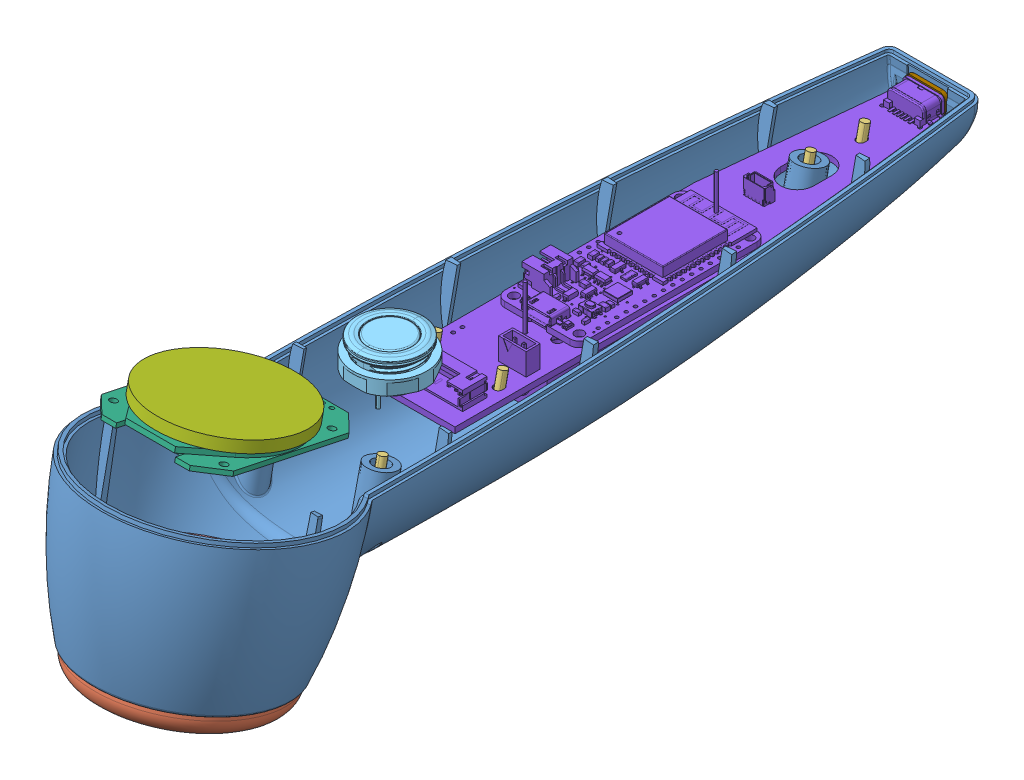
SolidWorks assembly PlasticScannerAssembly, configuration Default. Lengths in mm.
Overall size (62.38 71.41 231.21).
20 component instances, 13 part files, 54 mates.
Components (placement in the parent):
- Bottom shell-1: Bottom shell [Default] at origin size (62.38 51.39 230.69)
- Top Shell-1: Top Shell [Default] at origin size (62 34.67 227.14) (hidden)
- D profile seal ring-1: D profile seal ring [Default] at (0 -28.8554 6.1334) x (-0.032569 0.207801 0.977629) z (0.999469 0.006772 0.031857) size (48 7 48)
- BN_20002_3148566_hexalobular_socket_pan_head_screw_2_2x6-1: BN_20002_3148566_hexalobular_socket_pan_head_screw_2_2x6 [Default] at (-17.145 -14.0085 12.9751) x (0 -0.978148 0.207912) z (-0.651464 -0.157738 -0.7421) size (7.61 4 4)
- BN_20002_3148566_hexalobular_socket_pan_head_screw_2_2x6-2: BN_20002_3148566_hexalobular_socket_pan_head_screw_2_2x6 [Default] at (14.351 -17.7843 -4.7891) x (0 -0.978148 0.207912) z (-0.207912 0.203368 0.956773) size (7.61 4 4)
- PCB KiCad v0.4-1: PCB KiCad v0.4 [Default] at (-0.254 -16.1472 2.9129) x (1 0 0) z (0 -0.978148 0.207912) size (49.12 49.12 11.99)
- Push_buttonSwitch_MCS16_ZNC_ZNC_PIN_02-1: Push_buttonSwitch_MCS16_ZNC_ZNC_PIN_02 [Default] at (0 8.2 -50) size (20 15.41 20)
- BN_20002_3148566_hexalobular_socket_pan_head_screw_2_2x6-3: BN_20002_3148566_hexalobular_socket_pan_head_screw_2_2x6 [Default] at (-16 0.6097 -30.7998) x (0 0.978148 -0.207912) z (-0.207912 -0.203368 -0.956773) size (7.61 4 4)
- BN_20002_3148566_hexalobular_socket_pan_head_screw_2_2x6-4: BN_20002_3148566_hexalobular_socket_pan_head_screw_2_2x6 [Default] at (16 0.6097 -30.7998) x (0 0.978148 -0.207912) z (-0.207912 -0.203368 -0.956773) size (7.61 4 4)
- BN_20002_3148566_hexalobular_socket_pan_head_screw_2_2x6-5: BN_20002_3148566_hexalobular_socket_pan_head_screw_2_2x6 [Default] at (0 -1.9651 -163.1568) x (0 0.978148 -0.207912) z (-0.710006 -0.14641 -0.688807) size (7.61 4 4)
- Screen GC9A01 128 tft-1: Screen GC9A01 128 tft [Default] at (0 21.3737 -5.2588) x (1 0 0) z (0 0.207912 0.978148) size (36 2.7 44)
- 3mm glass-1: 3mm glass [Default] at (0 22.9865 -4.8859) x (0.980992 0.040345 0.189807) z (-0.194047 0.20396 0.959555) size (38 3 38)
- ControllerBoard -02-12-2022-2: ControllerBoard -02-12-2022 [Default] at (110.65 -2.1 -20.2) x (-1 0 0) z (0 1 0) size (25 142.1 26.9)
- CX60-24S-1000-C--3DModel-STEP-1-1: CX60-24S-1000-C--3DModel-STEP-1 [Default] at (4.05 7.135 -1179.513) x (0 0 1) z (0 -1 0) size (1000.01 12.36 6.51) (hidden)
- USB gasket-1: USB gasket [Default] at (0 1.25 -196.9) size (11 5.5 1.5)
- Lower glass-1: Lower glass [Default] at (0 -23.4755 4.9899) x (1 0 0) z (0 0.207912 0.978148) size (25 2 25)
- Lower O ring-1: Lower O ring [Default] at (0 -21.3236 4.5325) x (0.999365 0.007406 0.034843) z (-0.035621 0.20778 0.977527) size (25 8.31 25)
- BN_20002_3148566_hexalobular_socket_pan_head_screw_2_2x6-6: BN_20002_3148566_hexalobular_socket_pan_head_screw_2_2x6 [Default] at (0 -2.5158 -177.8637) x (0 0.978148 -0.207912) z (-0.710006 -0.14641 -0.688807) size (7.61 4 4)
- BN_20002_3148566_hexalobular_socket_pan_head_screw_2_2x6-7: BN_20002_3148566_hexalobular_socket_pan_head_screw_2_2x6 [Default] at (9 -2.5158 -70.5179) x (0 0.978148 -0.207912) z (-0.710006 -0.14641 -0.688807) size (7.61 4 4)
- BN_20002_3148566_hexalobular_socket_pan_head_screw_2_2x6-8: BN_20002_3148566_hexalobular_socket_pan_head_screw_2_2x6 [Default] at (-9 -2.5158 -70.5179) x (0 0.978148 -0.207912) z (-0.710006 -0.14641 -0.688807) size (7.61 4 4)
Mates (geometry in assembly coordinates):
- Coincident1: coincident aligned: plane of Bottom shell-1 through (0 0 0) normal (0 0 1)
- Coincident2: coincident aligned: plane of Top Shell-1 through (0 0 0) normal (0 0 1)
- Coincident3: coincident aligned: plane of Bottom shell-1 through (0 0 0) normal (0 1 0)
- Coincident4: coincident aligned: plane of Top Shell-1 through (0 0 0) normal (0 1 0)
- Coincident5: coincident aligned: plane of Bottom shell-1 through (0 0 0) normal (1 0 0)
- Coincident6: coincident aligned: plane of Top Shell-1 through (0 0 0) normal (1 0 0)
- Concentric5: concentric aligned: cone of Bottom shell-1 through (-17.145 -16.5516 13.5156) axis (0 -0.978148 0.207912); cylinder of BN_20002_3148566_hexalobular_socket_pan_head_screw_2_2x6-1 through (-17.145 -19.8773 14.2225) axis (0 -0.978148 0.207912) radius 1.1
- Concentric7: concentric anti-aligned: circle of Bottom shell-1; circle of PCB KiCad v0.4-1
- Concentric8: concentric aligned: cylinder of BN_20002_3148566_hexalobular_socket_pan_head_screw_2_2x6-2 through (14.351 -23.6532 -3.5416) axis (0 -0.978148 0.207912) radius 1.1; circle of PCB KiCad v0.4-1
- Coincident13: coincident anti-aligned: plane of Bottom shell-1 through (0 -19.3494 -4.4564) normal (0 0.978148 -0.207912); plane of PCB KiCad v0.4-1 through (0 -17.6067 3.7424) normal (0 -0.978148 0.207912)
- Coincident14: coincident anti-aligned: circle of BN_20002_3148566_hexalobular_socket_pan_head_screw_2_2x6-2; plane of PCB KiCad v0.4-1 through (0 -16.0416 3.4098) normal (0 0.978148 -0.207912)
- Coincident15: coincident anti-aligned: circle of BN_20002_3148566_hexalobular_socket_pan_head_screw_2_2x6-1; plane of PCB KiCad v0.4-1 through (0 -16.0416 3.4098) normal (0 0.978148 -0.207912)
- Concentric9: concentric anti-aligned: circle of Bottom shell-1; circle of PCB KiCad v0.4-1
- Concentric11: concentric aligned: cylinder of Bottom shell-1 through (0 -34.3669 36.4416) axis (0 0.978148 -0.207912) radius 1.15; cylinder of BN_20002_3148567_hexalobular_socket_pan_head_screw_2_2x8-1 through (0 20.1086 24.8625) axis (0 0.978148 -0.207912) radius 1.1
- Coincident18: coincident anti-aligned: plane of Bottom shell-1 through (0 6.358 -1.3514) normal (0 -0.978148 0.207912); circle of BN_20002_3148567_hexalobular_socket_pan_head_screw_2_2x8-1
- Distance1: distance = 0.5 mm anti-aligned: plane of Top Shell-1 through (0 16.5 0) normal (0 1 0); plane of Push_buttonSwitch_MCS16_ZNC_ZNC_PIN_02-1 through (0 17 -58) normal (0 -1 0)
- Coincident24: coincident aligned: plane of Push_buttonSwitch_MCS16_ZNC_ZNC_PIN_02-1 through (0 8.2 -50) normal (1 0 0)
- Coincident27: coincident: line of Top Shell-1 through (-2.506 14 -57.65) axis (1 0 0); line of Push_buttonSwitch_MCS16_ZNC_ZNC_PIN_02-1 through (0 16.95 -57.2) axis (0 -1 0)
- Concentric12: concentric aligned: circle of Top Shell-1; cylinder of Push_buttonSwitch_MCS16_ZNC_ZNC_PIN_02-1 through (0 8.2 -50) axis (0 1 0) radius 9
- Concentric13: concentric aligned: cone of Bottom shell-1 through (0 -1.9651 -163.1568) axis (0 0.978148 -0.207912); cylinder of BN_20002_3148566_hexalobular_socket_pan_head_screw_2_2x6-5 through (0 3.9037 -164.4043) axis (0 0.978148 -0.207912) radius 1.1
- Coincident28: coincident anti-aligned: plane of Bottom shell-1 through (0 31.3007 -6.6532) normal (0 -0.978148 0.207912); plane of BN_20002_3148566_hexalobular_socket_pan_head_screw_2_2x6-5 through (1.4084 -2.2604 -164.5458) normal (0 0.978148 -0.207912)
- Concentric14: concentric aligned: cone of Bottom shell-1 through (16 0.6097 -30.7998) axis (0 0.978148 -0.207912); cylinder of BN_20002_3148566_hexalobular_socket_pan_head_screw_2_2x6-4 through (16 6.4786 -32.0473) axis (0 0.978148 -0.207912) radius 1.1
- Coincident29: coincident anti-aligned: plane of Bottom shell-1 through (0 6.847 -1.4554) normal (0 -0.978148 0.207912); circle of BN_20002_3148566_hexalobular_socket_pan_head_screw_2_2x6-4
- Concentric15: concentric aligned: cone of Bottom shell-1 through (-16 0.6097 -30.7998) axis (0 0.978148 -0.207912); cylinder of BN_20002_3148566_hexalobular_socket_pan_head_screw_2_2x6-3 through (-16 6.4786 -32.0473) axis (0 0.978148 -0.207912) radius 1.1
- Coincident30: coincident anti-aligned: plane of Bottom shell-1 through (0 6.847 -1.4554) normal (0 -0.978148 0.207912); circle of BN_20002_3148566_hexalobular_socket_pan_head_screw_2_2x6-3
- Coincident40: coincident aligned: plane of Screen GC9A01 128 tft-1 through (0 21.3737 -5.2588) normal (1 0 0)
- Concentric21: concentric aligned: cone of Top Shell-1 through (-15 21.8241 -19.974) axis (0 0.978148 -0.207912); circle of Screen GC9A01 128 tft-1
- Coincident53: coincident anti-aligned: plane of Top Shell-1 through (0 -0.5 0) normal (0 -1 0); plane of ControllerBoard - 24-11-2022-1 through (0 0 -114.9863) normal (0 1 0)
- Parallel1: parallel anti-aligned: plane of ControllerBoard - 24-11-2022-1 through (-12.5 -1.6 -34.2242) normal (-1 0 0)
- Symmetric4: symmetric aligned: plane of ControllerBoard - 24-11-2022-1 through (-12.5 -1.6 -34.2242) normal (-1 0 0); plane of ControllerBoard - 24-11-2022-1 through (12.5 -1.6 -144.2242) normal (1 0 0)
- Parallel2: parallel anti-aligned: plane of ControllerBoard -02-12-2022-2 through (0 -2.1 -125.8975) normal (0 -1 0)
- Coincident55: coincident anti-aligned: plane of Top Shell-1 through (0 -0.5 0) normal (0 -1 0); plane of ControllerBoard -02-12-2022-2 through (0 -0.5 -125.8975) normal (0 1 0)
- Tangent1: tangent: curve of ?
- Width1: width anti-aligned: plane of CX60-24S-1000-C--3DModel-STEP-1-1 through (3.885 -2 -219.4838) normal (0 -1 0); plane of Bottom shell-1 through (-3.885 4.5 -219.4838) normal (0 1 0); plane of CX60-24S-1000-C--3DModel-STEP-1-1 through (0 -0.43 31.3023) normal (0 1 0); plane of Bottom shell-1 through (0 2.93 31.3023) normal (0 -1 0)
- Width2: width aligned: plane of CX60-24S-1000-C--3DModel-STEP-1-1 through (3.415 1.6948 -192.5402) normal (-1 0 0); plane of Bottom shell-1 through (-3.415 0.8252 -192.5402) normal (1 0 0); plane of CX60-24S-1000-C--3DModel-STEP-1-1 through (4.57 0 31.3023) normal (-1 0 0); plane of Bottom shell-1 through (-4.57 0 31.3023) normal (1 0 0)
- Distance5: distance = 0.5 mm anti-aligned: plane of Bottom shell-1 through (3.9 2.4 -196.4) normal (0 0 1); plane of USB gasket-1 through (-3.9 0.1 -196.9) normal (0 0 -1)
- Concentric35: concentric aligned: cylinder of Bottom shell-1 through (-3.14 1 31.3023) axis (0 0 -1) radius 1.43; cylinder of USB gasket-1 through (-3.14 1 -195.4) axis (0 0 -1) radius 1.43
- Concentric36: concentric aligned: cylinder of Bottom shell-1 through (3.14 1 31.3023) axis (0 0 -1) radius 1.43; cylinder of USB gasket-1 through (3.14 1 -195.4) axis (0 0 -1) radius 1.43
- Coincident59: coincident: plane of ControllerBoard -02-12-2022-2 through (0 -1.15 -195.4) normal (0 0 -1); point of USB gasket-1
- Coincident60: coincident: point of ControllerBoard -02-12-2022-2; plane of CX60-24S-1000-C--3DModel-STEP-1-1 through (4.0312 0.2687 -192.5) normal (0 0 1)
- Parallel3: parallel anti-aligned: plane of ControllerBoard -02-12-2022-2 through (110.65 -2.1 -20.2) normal (-1 0 0)
- Concentric37: concentric anti-aligned: cylinder of Bottom shell-1 through (0 -28.8554 6.1334) axis (0 -0.978148 0.207912) radius 24; cylinder of D profile seal ring-1 through (0 -28.8554 6.1334) axis (0 0.978148 -0.207912) radius 24
- Coincident61: coincident anti-aligned: plane of Bottom shell-1 through (0 -28.8554 6.1334) normal (0 -0.978148 0.207912); plane of D profile seal ring-1 through (-0.035 -31.974 -8.5388) normal (0 0.978148 -0.207912)
- Concentric38: concentric aligned: cone of Bottom shell-1 through (0 -21.3236 4.5325) axis (0 0.978148 -0.207912); line of Lower O ring-1 through (0 -21.3236 4.5325) axis (0 0.978148 -0.207912)
- Concentric39: concentric anti-aligned: cone of Bottom shell-1 through (0 -21.3236 4.5325) axis (0 0.978148 -0.207912); cylinder of Lower glass-1 through (0 -21.5192 4.5741) axis (0 -0.978148 0.207912) radius 12.5
- Coincident63: coincident anti-aligned: plane of Bottom shell-1 through (0 -21.3236 4.5325) normal (0 -0.978148 0.207912); plane of Lower O ring-1 through (0 -21.3236 4.5325) normal (0 0.978148 -0.207912)
- Coincident62: coincident aligned: plane of Bottom shell-1 through (0 -23.4755 4.9899) normal (0 0.978148 -0.207912); circle of Lower glass-1
- Symmetric5: symmetric aligned: plane of ControllerBoard -02-12-2022-2 through (12.5 -2.1 -145.2) normal (1 0 0); plane of ControllerBoard -02-12-2022-2 through (-12.5 -2.1 -55.2) normal (-1 0 0)
- Concentric40: concentric aligned: cone of Top Shell-1 through (9 1.2005 -71.3078) axis (0 0.978148 -0.207912); cylinder of BN_20002_3148566_hexalobular_socket_pan_head_screw_2_2x6-7 through (9 3.3531 -71.7654) axis (0 0.978148 -0.207912) radius 1.1
- Concentric41: concentric aligned: cone of Top Shell-1 through (-9 1.2005 -71.3078) axis (0 0.978148 -0.207912); cylinder of BN_20002_3148566_hexalobular_socket_pan_head_screw_2_2x6-8 through (-9 3.3531 -71.7654) axis (0 0.978148 -0.207912) radius 1.1
- Concentric42: concentric aligned: cone of Top Shell-1 through (0 0.889 -178.5874) axis (0 0.978148 -0.207912); cylinder of BN_20002_3148566_hexalobular_socket_pan_head_screw_2_2x6-6 through (0 3.3531 -179.1111) axis (0 0.978148 -0.207912) radius 1.1
- Tangent2: tangent: plane of ControllerBoard -02-12-2022-2 through (0 -2.1 -125.8975) normal (0 -1 0); circle of BN_20002_3148566_hexalobular_socket_pan_head_screw_2_2x6-6
- Tangent3: tangent: plane of ControllerBoard -02-12-2022-2 through (0 -2.1 -125.8975) normal (0 -1 0); circle of BN_20002_3148566_hexalobular_socket_pan_head_screw_2_2x6-7
- Tangent4: tangent: plane of ControllerBoard -02-12-2022-2 through (0 -2.1 -125.8975) normal (0 -1 0); circle of BN_20002_3148566_hexalobular_socket_pan_head_screw_2_2x6-8
